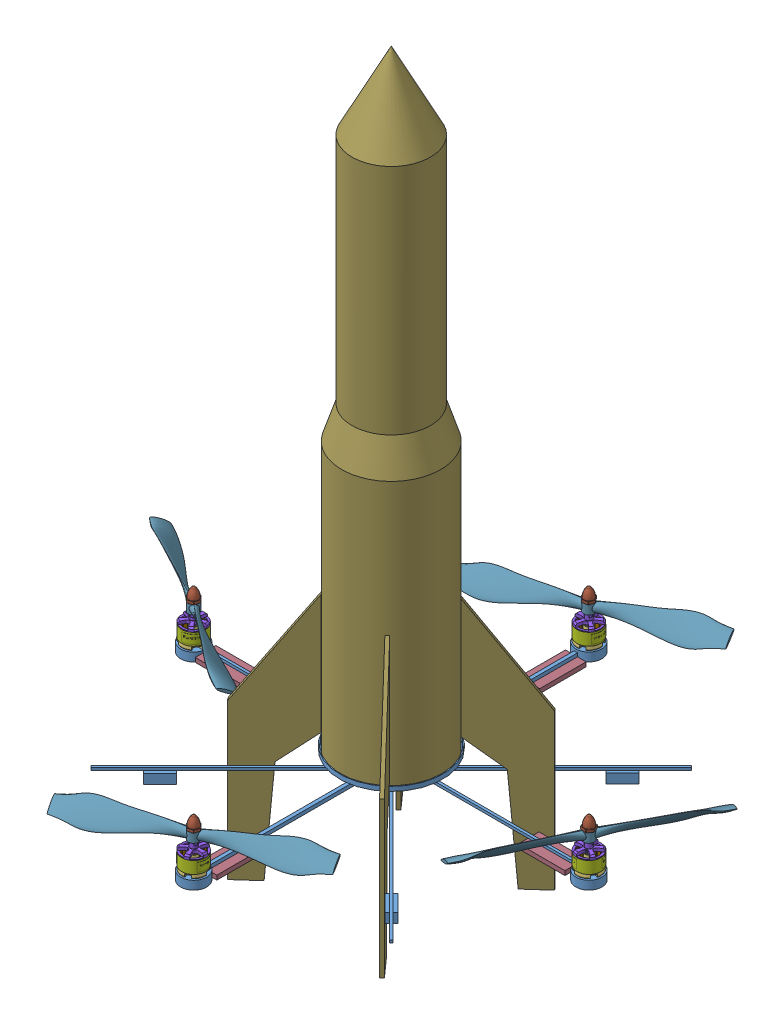
SolidWorks assembly Esamblaje Cohete2.0, configuration Predeterminado. Lengths in mm.
Overall size (638.66 842.22 591.08).
107 component instances, 15 part files, 40 mates.
Components (placement in the parent):
- Base pila2.0-1: Base pila2.0 [Predeterminado] at (0.2487 0 -0.1681) x (0.339851 0 -0.940479) z (0.940479 0 0.339851) size (461.66 176.4 461.66)
- Batería-1: Batería [Predeterminado] at (-0.6009 5 2.1831) x (0.339851 0 -0.940479) z (0.940479 0 0.339851) size (45 125 28)
- Assembly-1: Assembly [Default] at (11.0135 -6.4568 -204.1581) x (-0.921604 0 0.388132) z (-0.388132 0 -0.921604) size (45.37 57.6 38.97)
  - Motor Casing-1: Motor Casing [Default] at (0.0476 0.0568 27.7) size (27.7 18.09 27.7)
  - Drive Shaft-1: Drive Shaft [Default] at (0.0476 25.2068 27.7) x (0 -1 0) z (-0.763091 0 -0.646291) size (26.25 3 3)
  - Electrical Windings-1: Electrical Windings [Default] at (0.0476 18.0568 27.7) x (1 0 -0.000785) z (-0.000785 0 -1) size (36.88 20.62 22) (hidden)
  - instrument ball bearing_68_iso-1: instrument ball bearing_68_iso [ISO 1224 - 390308 - R,8,DE,NC,8_68] at (0.0476 2.0568 27.7) x (0 -1 0) z (0.020466 0 0.999791) size (4 8 8)
  - e-ring external retaining ring_wti-4: e-ring external retaining ring_wti [Truarc X5133-14 - S0.14] at (0.0476 0.0355 27.7) x (0.994275 0 -0.106853) z (0 1 0) size (5.26 4.55 0.38)
  - Rotor Cover-1: Rotor Cover [Default] at (0.0476 5.0568 27.7) x (0.291228 0 -0.956654) z (0.956654 0 0.291228) size (27.65 14 28.06)
  - Rotor-1: Rotor [Default] at (0.0476 14.5568 27.7) x (-0.763091 0 -0.646291) z (0.646291 0 -0.763091) size (27.65 31.18 27.65)
  - Magnet-1: Magnet [Default] at (7.7444 12.0568 37.9586) x (0.799891 0 -0.600146) z (-0.600146 0 -0.799891) size (4 12 1.6)
  - Magnet-2: Magnet [Default] at (2.5312 12.0568 40.2822) x (0.98107 0 -0.193653) z (-0.193653 0 -0.98107) size (4 12 1.6)
  - Magnet-3: Magnet [Default] at (-3.174 12.0568 40.1138) x (0.967937 0 0.251195) z (0.251195 0 -0.967937) size (4 12 1.6)
  - Magnet-4: Magnet [Default] at (-8.2411 12.0568 37.4866) x (0.763091 0 0.646291) z (0.646291 0 -0.763091) size (4 12 1.6)
  - Magnet-5: Magnet [Default] at (-11.6666 12.0568 32.9211) x (0.407106 0 0.913381) z (0.913381 0 -0.407106) size (4 12 1.6)
  - Magnet-6: Magnet [Default] at (-12.7719 12.0568 27.3215) x (-0.029511 0 0.999564) z (0.999564 0 0.029511) size (4 12 1.6)
  - Magnet-7: Magnet [Default] at (-11.3381 12.0568 21.7969) x (-0.460283 0 0.887772) z (0.887772 0 0.460283) size (4 12 1.6)
  - Magnet-8: Magnet [Default] at (-7.6493 12.0568 17.4414) x (-0.799891 0 0.600146) z (0.600146 0 0.799891) size (4 12 1.6)
  - Magnet-9: Magnet [Default] at (-2.4361 12.0568 15.1178) x (-0.98107 0 0.193653) z (0.193653 0 0.98107) size (4 12 1.6)
  - Magnet-10: Magnet [Default] at (3.2691 12.0568 15.2862) x (-0.967937 0 -0.251195) z (-0.251195 0 0.967937) size (4 12 1.6)
  - Magnet-11: Magnet [Default] at (8.3362 12.0568 17.9134) x (-0.763091 0 -0.646291) z (-0.646291 0 0.763091) size (4 12 1.6)
  - Magnet-12: Magnet [Default] at (11.7617 12.0568 22.4789) x (-0.407106 0 -0.913381) z (-0.913381 0 0.407106) size (4 12 1.6)
  - Magnet-13: Magnet [Default] at (12.867 12.0568 28.0785) x (0.029511 0 -0.999564) z (-0.999564 0 -0.029511) size (4 12 1.6)
  - Magnet-14: Magnet [Default] at (11.4332 12.0568 33.6031) x (0.460283 0 -0.887772) z (-0.887772 0 -0.460283) size (4 12 1.6)
  - Stopper Screw-1: Stopper Screw [Default] at (-0.5987 21.8426 28.4631) x (-0.646291 0 0.763091) z (-0.763091 0 -0.646291) size (2.64 2.54 2.89)
  - Nut-2: Nut [Default] at (0.0983 41.5568 27.7396) x (-0.763091 0 -0.646291) z (0.646291 0 -0.763091) size (12.11 14.31 13.7)
- Assembly-2: Assembly [Default] at (205.0166 -6.4568 -12.6729) x (0.451875 0 -0.892081) z (0.892081 0 0.451875) size (45.37 57.6 38.97)
  - Motor Casing-1: Motor Casing [Default] at (0.0476 0.0568 27.7) size (27.7 18.09 27.7)
  - Drive Shaft-1: Drive Shaft [Default] at (0.0476 25.2068 27.7) x (0 -1 0) z (-0.763091 0 -0.646291) size (26.25 3 3)
  - Electrical Windings-1: Electrical Windings [Default] at (0.0476 18.0568 27.7) x (1 0 -0.000785) z (-0.000785 0 -1) size (36.88 20.62 22) (hidden)
  - instrument ball bearing_68_iso-1: instrument ball bearing_68_iso [ISO 1224 - 390308 - R,8,DE,NC,8_68] at (0.0476 2.0568 27.7) x (0 -1 0) z (0.020466 0 0.999791) size (4 8 8)
  - e-ring external retaining ring_wti-4: e-ring external retaining ring_wti [Truarc X5133-14 - S0.14] at (0.0476 0.0355 27.7) x (0.994275 0 -0.106853) z (0 1 0) size (5.26 4.55 0.38)
  - Rotor Cover-1: Rotor Cover [Default] at (0.0476 5.0568 27.7) x (0.291228 0 -0.956654) z (0.956654 0 0.291228) size (27.65 14 28.06)
  - Rotor-1: Rotor [Default] at (0.0476 14.5568 27.7) x (-0.763091 0 -0.646291) z (0.646291 0 -0.763091) size (27.65 31.18 27.65)
  - Magnet-1: Magnet [Default] at (7.7444 12.0568 37.9586) x (0.799891 0 -0.600146) z (-0.600146 0 -0.799891) size (4 12 1.6)
  - Magnet-2: Magnet [Default] at (2.5312 12.0568 40.2822) x (0.98107 0 -0.193653) z (-0.193653 0 -0.98107) size (4 12 1.6)
  - Magnet-3: Magnet [Default] at (-3.174 12.0568 40.1138) x (0.967937 0 0.251195) z (0.251195 0 -0.967937) size (4 12 1.6)
  - Magnet-4: Magnet [Default] at (-8.2411 12.0568 37.4866) x (0.763091 0 0.646291) z (0.646291 0 -0.763091) size (4 12 1.6)
  - Magnet-5: Magnet [Default] at (-11.6666 12.0568 32.9211) x (0.407106 0 0.913381) z (0.913381 0 -0.407106) size (4 12 1.6)
  - Magnet-6: Magnet [Default] at (-12.7719 12.0568 27.3215) x (-0.029511 0 0.999564) z (0.999564 0 0.029511) size (4 12 1.6)
  - Magnet-7: Magnet [Default] at (-11.3381 12.0568 21.7969) x (-0.460283 0 0.887772) z (0.887772 0 0.460283) size (4 12 1.6)
  - Magnet-8: Magnet [Default] at (-7.6493 12.0568 17.4414) x (-0.799891 0 0.600146) z (0.600146 0 0.799891) size (4 12 1.6)
  - Magnet-9: Magnet [Default] at (-2.4361 12.0568 15.1178) x (-0.98107 0 0.193653) z (0.193653 0 0.98107) size (4 12 1.6)
  - Magnet-10: Magnet [Default] at (3.2691 12.0568 15.2862) x (-0.967937 0 -0.251195) z (-0.251195 0 0.967937) size (4 12 1.6)
  - Magnet-11: Magnet [Default] at (8.3362 12.0568 17.9134) x (-0.763091 0 -0.646291) z (-0.646291 0 0.763091) size (4 12 1.6)
  - Magnet-12: Magnet [Default] at (11.7617 12.0568 22.4789) x (-0.407106 0 -0.913381) z (-0.913381 0 0.407106) size (4 12 1.6)
  - Magnet-13: Magnet [Default] at (12.867 12.0568 28.0785) x (0.029511 0 -0.999564) z (-0.999564 0 -0.029511) size (4 12 1.6)
  - Magnet-14: Magnet [Default] at (11.4332 12.0568 33.6031) x (0.460283 0 -0.887772) z (-0.887772 0 -0.460283) size (4 12 1.6)
  - Stopper Screw-1: Stopper Screw [Default] at (-0.5987 21.8426 28.4631) x (-0.646291 0 0.763091) z (-0.763091 0 -0.646291) size (2.64 2.54 2.89)
  - Nut-2: Nut [Default] at (0.0983 41.5568 27.7396) x (-0.763091 0 -0.646291) z (0.646291 0 -0.763091) size (12.11 14.31 13.7)
- Assembly-3: Assembly [Default] at (-11.3773 -6.4568 204.2038) x (0.907871 0 -0.419249) z (0.419249 0 0.907871) size (45.37 57.6 38.97)
  - Motor Casing-1: Motor Casing [Default] at (0.0476 0.0568 27.7) size (27.7 18.09 27.7)
  - Drive Shaft-1: Drive Shaft [Default] at (0.0476 25.2068 27.7) x (0 -1 0) z (-0.763091 0 -0.646291) size (26.25 3 3)
  - Electrical Windings-1: Electrical Windings [Default] at (0.0476 18.0568 27.7) x (1 0 -0.000785) z (-0.000785 0 -1) size (36.88 20.62 22) (hidden)
  - instrument ball bearing_68_iso-1: instrument ball bearing_68_iso [ISO 1224 - 390308 - R,8,DE,NC,8_68] at (0.0476 2.0568 27.7) x (0 -1 0) z (0.020466 0 0.999791) size (4 8 8)
  - e-ring external retaining ring_wti-4: e-ring external retaining ring_wti [Truarc X5133-14 - S0.14] at (0.0476 0.0355 27.7) x (0.994275 0 -0.106853) z (0 1 0) size (5.26 4.55 0.38)
  - Rotor Cover-1: Rotor Cover [Default] at (0.0476 5.0568 27.7) x (0.291228 0 -0.956654) z (0.956654 0 0.291228) size (27.65 14 28.06)
  - Rotor-1: Rotor [Default] at (0.0476 14.5568 27.7) x (-0.763091 0 -0.646291) z (0.646291 0 -0.763091) size (27.65 31.18 27.65)
  - Magnet-1: Magnet [Default] at (7.7444 12.0568 37.9586) x (0.799891 0 -0.600146) z (-0.600146 0 -0.799891) size (4 12 1.6)
  - Magnet-2: Magnet [Default] at (2.5312 12.0568 40.2822) x (0.98107 0 -0.193653) z (-0.193653 0 -0.98107) size (4 12 1.6)
  - Magnet-3: Magnet [Default] at (-3.174 12.0568 40.1138) x (0.967937 0 0.251195) z (0.251195 0 -0.967937) size (4 12 1.6)
  - Magnet-4: Magnet [Default] at (-8.2411 12.0568 37.4866) x (0.763091 0 0.646291) z (0.646291 0 -0.763091) size (4 12 1.6)
  - Magnet-5: Magnet [Default] at (-11.6666 12.0568 32.9211) x (0.407106 0 0.913381) z (0.913381 0 -0.407106) size (4 12 1.6)
  - Magnet-6: Magnet [Default] at (-12.7719 12.0568 27.3215) x (-0.029511 0 0.999564) z (0.999564 0 0.029511) size (4 12 1.6)
  - Magnet-7: Magnet [Default] at (-11.3381 12.0568 21.7969) x (-0.460283 0 0.887772) z (0.887772 0 0.460283) size (4 12 1.6)
  - Magnet-8: Magnet [Default] at (-7.6493 12.0568 17.4414) x (-0.799891 0 0.600146) z (0.600146 0 0.799891) size (4 12 1.6)
  - Magnet-9: Magnet [Default] at (-2.4361 12.0568 15.1178) x (-0.98107 0 0.193653) z (0.193653 0 0.98107) size (4 12 1.6)
  - Magnet-10: Magnet [Default] at (3.2691 12.0568 15.2862) x (-0.967937 0 -0.251195) z (-0.251195 0 0.967937) size (4 12 1.6)
  - Magnet-11: Magnet [Default] at (8.3362 12.0568 17.9134) x (-0.763091 0 -0.646291) z (-0.646291 0 0.763091) size (4 12 1.6)
  - Magnet-12: Magnet [Default] at (11.7617 12.0568 22.4789) x (-0.407106 0 -0.913381) z (-0.913381 0 0.407106) size (4 12 1.6)
  - Magnet-13: Magnet [Default] at (12.867 12.0568 28.0785) x (0.029511 0 -0.999564) z (-0.999564 0 -0.029511) size (4 12 1.6)
  - Magnet-14: Magnet [Default] at (11.4332 12.0568 33.6031) x (0.460283 0 -0.887772) z (-0.887772 0 -0.460283) size (4 12 1.6)
  - Stopper Screw-1: Stopper Screw [Default] at (-0.5987 21.8426 28.4631) x (-0.646291 0 0.763091) z (-0.763091 0 -0.646291) size (2.64 2.54 2.89)
  - Nut-2: Nut [Default] at (0.0983 41.5568 27.7396) x (-0.763091 0 -0.646291) z (0.646291 0 -0.763091) size (12.11 14.31 13.7)
- Assembly-4: Assembly [Default] at (-214.4771 -6.4568 -23.5688) x (0.844969 0 0.534815) z (-0.534815 0 0.844969) size (45.37 57.6 38.97)
  - Motor Casing-1: Motor Casing [Default] at (0.0476 0.0568 27.7) size (27.7 18.09 27.7)
  - Drive Shaft-1: Drive Shaft [Default] at (0.0476 25.2068 27.7) x (0 -1 0) z (-0.763091 0 -0.646291) size (26.25 3 3)
  - Electrical Windings-1: Electrical Windings [Default] at (0.0476 18.0568 27.7) x (1 0 -0.000785) z (-0.000785 0 -1) size (36.88 20.62 22) (hidden)
  - instrument ball bearing_68_iso-1: instrument ball bearing_68_iso [ISO 1224 - 390308 - R,8,DE,NC,8_68] at (0.0476 2.0568 27.7) x (0 -1 0) z (0.020466 0 0.999791) size (4 8 8)
  - e-ring external retaining ring_wti-4: e-ring external retaining ring_wti [Truarc X5133-14 - S0.14] at (0.0476 0.0355 27.7) x (0.994275 0 -0.106853) z (0 1 0) size (5.26 4.55 0.38)
  - Rotor Cover-1: Rotor Cover [Default] at (0.0476 5.0568 27.7) x (0.291228 0 -0.956654) z (0.956654 0 0.291228) size (27.65 14 28.06)
  - Rotor-1: Rotor [Default] at (0.0476 14.5568 27.7) x (-0.763091 0 -0.646291) z (0.646291 0 -0.763091) size (27.65 31.18 27.65)
  - Magnet-1: Magnet [Default] at (7.7444 12.0568 37.9586) x (0.799891 0 -0.600146) z (-0.600146 0 -0.799891) size (4 12 1.6)
  - Magnet-2: Magnet [Default] at (2.5312 12.0568 40.2822) x (0.98107 0 -0.193653) z (-0.193653 0 -0.98107) size (4 12 1.6)
  - Magnet-3: Magnet [Default] at (-3.174 12.0568 40.1138) x (0.967937 0 0.251195) z (0.251195 0 -0.967937) size (4 12 1.6)
  - Magnet-4: Magnet [Default] at (-8.2411 12.0568 37.4866) x (0.763091 0 0.646291) z (0.646291 0 -0.763091) size (4 12 1.6)
  - Magnet-5: Magnet [Default] at (-11.6666 12.0568 32.9211) x (0.407106 0 0.913381) z (0.913381 0 -0.407106) size (4 12 1.6)
  - Magnet-6: Magnet [Default] at (-12.7719 12.0568 27.3215) x (-0.029511 0 0.999564) z (0.999564 0 0.029511) size (4 12 1.6)
  - Magnet-7: Magnet [Default] at (-11.3381 12.0568 21.7969) x (-0.460283 0 0.887772) z (0.887772 0 0.460283) size (4 12 1.6)
  - Magnet-8: Magnet [Default] at (-7.6493 12.0568 17.4414) x (-0.799891 0 0.600146) z (0.600146 0 0.799891) size (4 12 1.6)
  - Magnet-9: Magnet [Default] at (-2.4361 12.0568 15.1178) x (-0.98107 0 0.193653) z (0.193653 0 0.98107) size (4 12 1.6)
  - Magnet-10: Magnet [Default] at (3.2691 12.0568 15.2862) x (-0.967937 0 -0.251195) z (-0.251195 0 0.967937) size (4 12 1.6)
  - Magnet-11: Magnet [Default] at (8.3362 12.0568 17.9134) x (-0.763091 0 -0.646291) z (-0.646291 0 0.763091) size (4 12 1.6)
  - Magnet-12: Magnet [Default] at (11.7617 12.0568 22.4789) x (-0.407106 0 -0.913381) z (-0.913381 0 0.407106) size (4 12 1.6)
  - Magnet-13: Magnet [Default] at (12.867 12.0568 28.0785) x (0.029511 0 -0.999564) z (-0.999564 0 -0.029511) size (4 12 1.6)
  - Magnet-14: Magnet [Default] at (11.4332 12.0568 33.6031) x (0.460283 0 -0.887772) z (-0.887772 0 -0.460283) size (4 12 1.6)
  - Stopper Screw-1: Stopper Screw [Default] at (-0.5987 21.8426 28.4631) x (-0.646291 0 0.763091) z (-0.763091 0 -0.646291) size (2.64 2.54 2.89)
  - Nut-2: Nut [Default] at (0.0983 41.5568 27.7396) x (-0.763091 0 -0.646291) z (0.646291 0 -0.763091) size (12.11 14.31 13.7)
- Carcasa Cohete-1: Carcasa Cohete [Predeterminado] at (0.2487 0 -0.1681) x (-0.666009 0 -0.745944) z (0.745944 0 -0.666009) size (269 842.22 269)
- Driver-1: Driver [Predeterminado] at (187.7487 -8.4 0.6409) x (0 0 1) z (1 0 0) size (24 5 54)
- Driver-2: Driver [Predeterminado] at (0.2003 -18.4 187.3319) size (24 5 54)
- Driver-3: Driver [Predeterminado] at (-187.2513 -13.4 0.9124) x (0 0 -1) z (1 0 0) size (24 5 54)
- Driver-4: Driver [Predeterminado] at (0.1343 -18.4 -187.6681) size (24 5 54)
- 13 INCH PROPELLER-1: 13 INCH PROPELLER [Default] at (0.279 29.35 229.3319) x (0.907871 0 -0.419249) z (0.419249 0 0.907871) size (250.01 25.97 24.54)
- 13 INCH PROPELLER-2: 13 INCH PROPELLER [Default] at (229.7487 29.35 -0.1984) x (-0.451875 0 0.892081) z (-0.892081 0 -0.451875) size (250.01 25.97 24.54)
- 13 INCH PROPELLER-3: 13 INCH PROPELLER [Default] at (-229.2513 29.35 -0.1378) x (-0.844969 0 -0.534815) z (0.534815 0 -0.844969) size (250.01 25.97 24.54)
- 13 INCH PROPELLER-4: 13 INCH PROPELLER [Default] at (0.2184 29.35 -229.6681) x (0.921604 0 -0.388132) z (0.388132 0 0.921604) size (250.01 25.97 24.54)
Mates (geometry in assembly coordinates):
- Coincidente1: coincident anti-aligned: plane of Base pila2.0-1 through (0.2487 5 -0.1681) normal (0 1 0); plane of Batería-1 through (-0.6009 5 2.1831) normal (0 -1 0)
- Coincidente2: coincident anti-aligned: plane of Base pila2.0-1 through (-12.918 75 -4.926) normal (0.940479 0 0.339851); plane of Batería-1 through (-6.121 130 -23.7356) normal (-0.940479 0 -0.339851)
- Coincidente3: coincident anti-aligned: plane of Base pila2.0-1 through (-8.2475 75 23.3439) normal (0.339851 0 -0.940479); plane of Batería-1 through (4.9192 130 28.1018) normal (-0.339851 0 0.940479)
- Concéntrica1: concentric anti-aligned: cylinder of Base pila2.0-1 through (0.2184 -16.4 -229.6681) axis (0 1 0) radius 15; cylinder of Assembly-1/Rotor Cover-1 through (0.2184 12.6 -229.6681) axis (0 -1 0) radius 13.825
- Coincidente4: coincident anti-aligned: plane of Base pila2.0-1 through (0.2184 -6.4 -229.6681) normal (0 1 0); plane of Assembly-1/Motor Casing-1 through (-11.1634 -6.4 -224.8747) normal (0 -1 0)
- Concéntrica2: concentric anti-aligned: cylinder of Base pila2.0-1 through (229.7487 -16.4 -0.1984) axis (0 1 0) radius 15; cylinder of Assembly-2/Rotor Cover-1 through (229.7487 12.6 -0.1984) axis (0 -1 0) radius 13.825
- Coincidente5: coincident anti-aligned: plane of Base pila2.0-1 through (229.7487 -6.4 -0.1984) normal (0 1 0); plane of Assembly-2/Motor Casing-1 through (235.3294 -6.4 -11.2156) normal (0 -1 0)
- Concéntrica3: concentric anti-aligned: cylinder of Assembly-3/Rotor Cover-1 through (0.279 12.6 229.3319) axis (0 -1 0) radius 13.825; cylinder of Base pila2.0-1 through (0.279 -16.4 229.3319) axis (0 1 0) radius 15
- Coincidente6: coincident anti-aligned: plane of Base pila2.0-1 through (0.279 -6.4 229.3319) normal (0 1 0); plane of Assembly-3/Motor Casing-1 through (11.4913 -6.4 224.1542) normal (0 -1 0)
- Concéntrica4: concentric anti-aligned: cylinder of Base pila2.0-1 through (-229.2513 -16.4 -0.1378) axis (0 1 0) radius 15; cylinder of Assembly-4/Rotor Cover-1 through (-229.2513 12.6 -0.1378) axis (0 -1 0) radius 13.825
- Coincidente7: coincident anti-aligned: plane of Base pila2.0-1 through (-229.2513 -6.4 -0.1378) normal (0 1 0); plane of Assembly-4/Motor Casing-1 through (-218.8159 -6.4 6.4672) normal (0 -1 0)
- Concéntrica6: concentric aligned: cylinder of Base pila2.0-1 through (0.2487 0 -0.1681) axis (0 -1 0) radius 59; cylinder of Carcasa Cohete-1 through (0.2487 310 -0.1681) axis (0 -1 0) radius 53.5
- Coincidente31: coincident anti-aligned: plane of Base pila2.0-1 through (0.2487 0 -0.1681) normal (0 1 0); plane of Carcasa Cohete-1 through (0.2487 0 -0.1681) normal (0 -1 0)
- Coincidente32: coincident aligned: plane of Base pila2.0-1 through (0.2487 0 -0.1681) normal (0 1 0)
- Coincidente33: coincident aligned: plane of Base pila2.0-1 through (0.2487 0 0) normal (0 0 1)
- Coincidente34: coincident aligned: plane of Base pila2.0-1 through (0 0 -0.1681) normal (1 0 0)
- Coincidente35: coincident anti-aligned: plane of Base pila2.0-1 through (214.7487 -8.4 1.5) normal (0 -1 0); plane of Driver-1 through (187.7487 -8.4 0.6409) normal (0 1 0)
- Paralelo11: parallel aligned: plane of Base pila2.0-1 through (214.7487 -5.4 -1.5) normal (0 0 -1); plane of Driver-1 through (214.7487 -13.4 -11.3591) normal (0 0 -1)
- Tangente1: tangent anti-aligned: cylinder of Base pila2.0-1 through (229.7487 -16.4 -0.1984) axis (0 1 0) radius 15; plane of Driver-1 through (214.7487 -13.4 12.6409) normal (1 0 0)
- Coincidente40: coincident anti-aligned: plane of Base pila2.0-1 through (-2 -13.4 214.3319) normal (0 -1 0); plane of Driver-2 through (0.2003 -13.4 187.3319) normal (0 1 0)
- Tangente3: tangent anti-aligned: cylinder of Base pila2.0-1 through (0.279 -16.4 229.3319) axis (0 1 0) radius 15; plane of Driver-2 through (12.2003 -13.4 214.3319) normal (0 0 1)
- Paralelo13: parallel aligned: plane of Base pila2.0-1 through (-2 -9.4 214.3319) normal (-1 0 0); plane of Driver-2 through (-11.7997 -13.4 214.3319) normal (-1 0 0)
- Coincidente42: coincident anti-aligned: plane of Base pila2.0-1 through (-214.2513 -8.4 1.5) normal (0 -1 0); plane of Driver-3 through (-187.2513 -8.4 0.9124) normal (0 1 0)
- Tangente4: tangent anti-aligned: cylinder of Base pila2.0-1 through (-229.2513 -16.4 -0.1378) axis (0 1 0) radius 15; plane of Driver-3 through (-214.2513 -8.4 -11.0876) normal (-1 0 0)
- Paralelo14: parallel aligned: plane of Base pila2.0-1 through (-214.2513 -5.4 1.5) normal (0 0 1); plane of Driver-3 through (-160.2513 -8.4 12.9124) normal (0 0 1)
- Coincidente44: coincident anti-aligned: plane of Base pila2.0-1 through (-2 -13.4 -214.6681) normal (0 -1 0); plane of Driver-4 through (0.1343 -13.4 -187.6681) normal (0 1 0)
- Tangente5: tangent anti-aligned: cylinder of Base pila2.0-1 through (0.2184 -16.4 -229.6681) axis (0 1 0) radius 15; plane of Driver-4 through (12.1343 -13.4 -214.6681) normal (0 0 -1)
- Paralelo15: parallel aligned: plane of Base pila2.0-1 through (-2 -9.4 -214.6681) normal (-1 0 0); plane of Driver-4 through (-11.8657 -13.4 -160.6681) normal (-1 0 0)
- Concéntrica7: concentric anti-aligned: cylinder of Assembly-3/Rotor-1 through (0.279 8.1 229.3319) axis (0 -1 0) radius 3; cylinder of 13 INCH PROPELLER-1 through (0.279 20.5112 229.3319) axis (0 1 0) radius 3.125
- Paralelo16: parallel aligned: plane of Assembly-3/Motor Casing-1 through (0.279 -6.4 229.3319) normal (0.419249 0 0.907871); plane of 13 INCH PROPELLER-1 through (0.279 29.35 229.3319) normal (0.419249 0 0.907871)
- Coincidente46: coincident anti-aligned: plane of Assembly-3/Nut-2 through (0.3417 35.1 229.3466) normal (0 -1 0); plane of 13 INCH PROPELLER-1 through (0.279 35.1 229.3319) normal (0 1 0)
- Concéntrica8: concentric anti-aligned: cylinder of Assembly-2/Rotor-1 through (229.7487 8.1 -0.1984) axis (0 -1 0) radius 3; cylinder of 13 INCH PROPELLER-2 through (229.7487 20.5112 -0.1984) axis (0 1 0) radius 3.125
- Paralelo17: parallel anti-aligned: plane of Assembly-2/Motor Casing-1 through (229.7487 -6.4 -0.1984) normal (0.892081 0 0.451875); plane of 13 INCH PROPELLER-2 through (229.7487 29.35 -0.1984) normal (-0.892081 0 -0.451875)
- Coincidente48: coincident anti-aligned: plane of Assembly-2/Nut-2 through (229.807 35.1 -0.2257) normal (0 -1 0); plane of 13 INCH PROPELLER-2 through (229.7487 35.1 -0.1984) normal (0 1 0)
- Concéntrica9: concentric anti-aligned: cylinder of Assembly-4/Rotor-1 through (-229.2513 8.1 -0.1378) axis (0 -1 0) radius 3; cylinder of 13 INCH PROPELLER-3 through (-229.2513 20.5112 -0.1378) axis (0 1 0) radius 3.125
- Coincidente49: coincident anti-aligned: plane of Assembly-4/Nut-2 through (-229.2296 35.1 -0.0772) normal (0 -1 0); plane of 13 INCH PROPELLER-3 through (-229.2513 35.1 -0.1378) normal (0 1 0)
- Paralelo18: parallel anti-aligned: plane of Assembly-4/Motor Casing-1 through (-229.2513 -6.4 -0.1378) normal (-0.534815 0 0.844969); plane of 13 INCH PROPELLER-3 through (-229.2513 29.35 -0.1378) normal (0.534815 0 -0.844969)
- Concéntrica10: concentric anti-aligned: cylinder of Assembly-1/Rotor-1 through (0.2184 8.1 -229.6681) axis (0 -1 0) radius 3; cylinder of 13 INCH PROPELLER-4 through (0.2184 20.5112 -229.6681) axis (0 1 0) radius 3.125
- Coincidente51: coincident anti-aligned: plane of Assembly-1/Nut-2 through (0.1563 35.1 -229.6849) normal (0 -1 0); plane of 13 INCH PROPELLER-4 through (0.2184 35.1 -229.6681) normal (0 1 0)
- Paralelo19: parallel anti-aligned: plane of Assembly-1/Motor Casing-1 through (0.2184 -6.4 -229.6681) normal (-0.388132 0 -0.921604); plane of 13 INCH PROPELLER-4 through (0.2184 29.35 -229.6681) normal (0.388132 0 0.921604)
